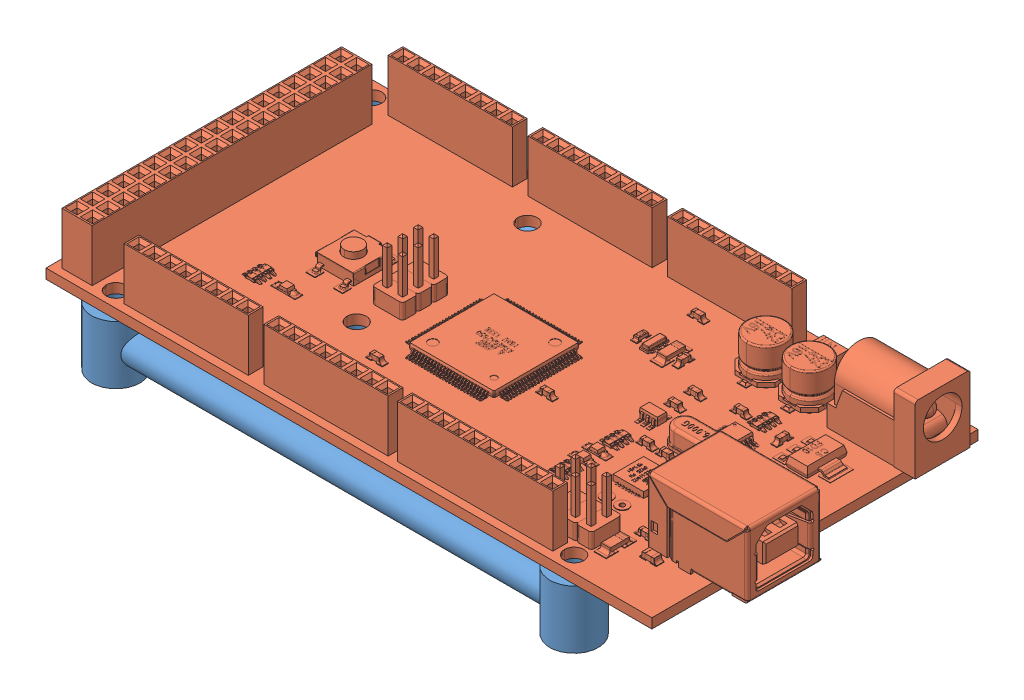
SolidWorks assembly Arduino MEGA Assembly, configuration Default. Lengths in mm.
Overall size (107.96 22.18 56.2).
2 component instances, 2 part files, 6 mates.
Components (placement in the parent):
- Arduino MEGA Mount-1: Arduino MEGA Mount [Default] at (55.245 9.525 0) x (-1 0 0) z (0 0 1) size (90.49 9.53 56.2)
- Arduino MEGA2650-1: Arduino MEGA2650 [Default] at (55.245 11.125 -26.67) x (0 0 -1) z (1 0 0) size (53.34 15.26 107.96)
Mates (geometry in assembly coordinates):
- Coincident1: coincident anti-aligned: plane of Arduino MEGA Mount-1 through (40.005 0 24.13) normal (0 -1 0)
- Coincident2: coincident aligned: plane of Arduino MEGA Mount-1 through (55.245 9.525 0) normal (0 0 1)
- Distance2: distance = 55.245 mm: plane of assembly through (0 0 0) normal (1 0 0); plane of assembly; plane of Arduino MEGA Mount-1 through (55.245 9.525 0) normal (-1 0 0)
- Coincident7: coincident: plane of Arduino MEGA Mount-1 through (41.275 9.525 -24.13) normal (0 1 0); plane of Arduino MEGA2650-1 through (55.245 9.525 -26.67) normal (0 -1 0)
- Concentric1: concentric: cylinder of Arduino MEGA Mount-1 through (-34.925 0 24.13) axis (0 1 0) radius 1.5875; cylinder of Arduino MEGA2650-1 through (-34.925 9.525 24.13) axis (0 1 0) radius 1.5875
- Concentric2: concentric aligned: cylinder of Arduino MEGA Mount-1 through (40.005 0 24.13) axis (0 1 0) radius 1.5875; cylinder of Arduino MEGA2650-1 through (40.005 9.525 24.13) axis (0 1 0) radius 1.5875
